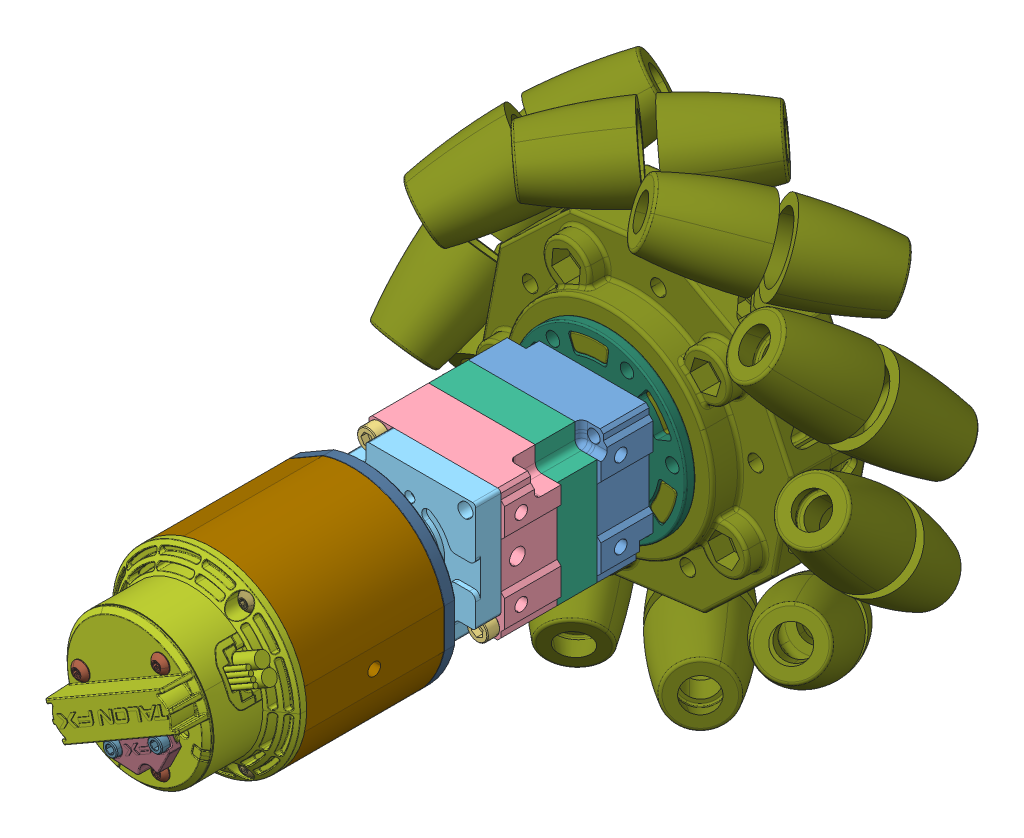
SolidWorks assembly LeftMotorStack, configuration Default. Lengths in mm.
Overall size (198.43 195.51 209.52).
34 component instances, 27 part files, 5 mates.
Components (placement in the parent):
- MotorStack-1: MotorStack [Default] at (-4.3094 29.1715 123.7803) size (81.62 81.39 192.35)
  - v2-VersaPlanetary-1stage-with-AM9015-20131031-1: v2-VersaPlanetary-1stage-with-AM9015-20131031 [Default] at (32.9453 91.261 18.2063) x (0 0 -1) z (0 1 0) size (95.9 44.45 42.1)
    - 217-2625-026 Rev1-1: 217-2625-026 Rev1 [Default] at (-6.5 22.225 0) x (0 -1 0) z (-1 0 0) size (44.45 42 18.13)
    - 217-2742-001 Rev4-1: 217-2742-001 Rev4 [Default] at (0.2002 22.225 0) x (1 0 0) z (0 -0.092627 0.995701) size (7 28 28)
    - 217-2742-001 Rev4-2: 217-2742-001 Rev4 [Default] at (8.2002 22.225 0) size (7 28 28)
    - 217-2625-017 Rev1_9714K61-1: 217-2625-017 Rev1_9714K61 [Default] at (7.42 22.3002 -0.342) x (0 0.56703 0.823697) z (0 -0.823697 0.56703) size (28.51 4.98 30.18)
    - 217-2625-003 Rev1-1: 217-2625-003 Rev1 [Default] at (7.4478 22.225 0) x (0 -1 0) z (1 0 0) size (17 17 64.12)
    - 217-2625-018 Rev1_98541A410-1: 217-2625-018 Rev1_98541A410 [Default] at (-0.7046 22.225 0) x (1 0 0) z (0 -0.017452 0.999848) size (1 19.6 17.4)
    - 832-1750-Ring-Gear-Screw_SSA0832-0500ZC-1: 832-1750-Ring-Gear-Screw_SSA0832-0500ZC [Default] at (-30.7 4.725 -17.5) x (0 0.997447 0.071411) z (0 -0.071411 0.997447) size (6.73 48.51 6.73)
    - 832-1750-Ring-Gear-Screw_SSA0832-0500ZC-2: 832-1750-Ring-Gear-Screw_SSA0832-0500ZC [Default] at (-30.7 39.725 17.5) x (0 0.005929 0.999982) z (0 -0.999982 0.005929) size (6.73 48.51 6.73)
    - 217-2625-025 Rev1-1: 217-2625-025 Rev1 [Default] at (-23.2 22.225 0) x (0 -1 0) z (-1 0 0) size (44.45 42 18)
    - 217-2822-004 Rev4-1: 217-2822-004 Rev4 [Default] at (-37.7 22.225 0) x (0 -1 0) z (-1 0 0) size (42 42 9.8)
    - 217-2820 Rev1_Public-1: 217-2820 Rev1_Public [Default] at (-4.6546 22.225 0) x (0 -0.456494 0.889726) z (-1 0 0)
      - 217-2625-100-1: 217-2625-100 [Default] at origin
    - 217-2816-001 Rev1-1: 217-2816-001 Rev1 [Default] at (-6.35 22.225 0) x (0 -1 0) z (1 0 0) size (42 42 14.5)
    - 217-4649-001 Rev1-1: 217-4649-001 Rev1 [Default] at (-20.046 22.225 0) x (0 -1 0) z (1 0 0) size (18 18 13)
    - 217-4649-007 Rev1_94105A824-1: 217-4649-007 Rev1_94105A824 [Default] at (-25.521 22.225 -6.7835) x (-0.996104 -0.088191 0) z (0 0 -1) size (4.83 4.83 4.9)
    - 217-2625-014 Rev2-1: 217-2625-014 Rev2 [Default] at (-24.7818 22.225 0) x (0 0 1) z (0 -1 0) size (8.01 7.5 7.94)
  - Falcon_500_Powered_by_Talon_FX_217-6515-1: Falcon_500_Powered_by_Talon_FX_217-6515 [Default] at (9.4877 97.4968 108.3478) x (1 0 0) z (0 0 -1) size (81.62 81.39 116.76)
    - Copy of 217-6515-Back 20190920^Falcon_500_Powered_by_Talon_FX_217-6515-1: Copy of 217-6515-Back 20190920^Falcon_500_Powered_by_Talon_FX_217-6515 [Default] at (1.2326 6.2358 -14.9619) size (60.06 60.12 79.55) (virtual)
    - Copy of Copy of 217-6515-201 Rev6^Falcon_500_Powered_by_Talon_FX_217-6515-1: Copy of Copy of 217-6515-201 Rev6^Falcon_500_Powered_by_Talon_FX_217-6515 [Default] at (1.2326 6.2358 50.6381) x (0.809017 0.587785 0) z (0 0 1) size (9.31 9.33 42.21) (virtual)
    - Copy of 217-6515-002 Rev6^Falcon_500_Powered_by_Talon_FX_217-6515-1: Copy of 217-6515-002 Rev6^Falcon_500_Powered_by_Talon_FX_217-6515 [Default] at (1.2326 6.2358 10.7381) x (0 -1 0) z (0 0 1) size (60 59.34 44.4) (virtual)
    - Copy of 217-6515-001 Rev6^Falcon_500_Powered_by_Talon_FX_217-6515-1: Copy of 217-6515-001 Rev6^Falcon_500_Powered_by_Talon_FX_217-6515 [Default] at (1.2326 6.2358 30.9381) x (0.5 0.866025 0) z (0 0 1) size (59.34 59.99 10) (virtual)
    - Copy of M3 BHTS-SECURE, Grade 8 Steel Rev1_SBTM3-24MMZB-SECURE^Falcon_500_Powered_by_Talon_FX_217-6515-1: Copy of M3 BHTS-SECURE, Grade 8 Steel Rev1_SBTM3-24MMZB-SECURE^Falcon_500_Powered_by_Talon_FX_217-6515 [Default] at (9.7324 20.9581 -38.0119) x (-0.923728 -0.383049 0) z (0 0 -1) size (5.69 5.69 25.65) (virtual)
    - Copy (2) of M3 BHTS-SECURE, Grade 8 Steel Rev1_SBTM3-24MMZB-SECURE^Falcon_500_Powered_by_Talon_FX_217-6515-2: Copy (2) of M3 BHTS-SECURE, Grade 8 Steel Rev1_SBTM3-24MMZB-SECURE^Falcon_500_Powered_by_Talon_FX_217-6515 [Default] at (-15.7672 6.2357 -38.0119) x (0.793594 -0.608447 0) z (0 0 -1) size (5.69 5.69 25.65) (virtual)
    - Copy (3) of M3 BHTS-SECURE, Grade 8 Steel Rev1_SBTM3-24MMZB-SECURE^Falcon_500_Powered_by_Talon_FX_217-6515-3: Copy (3) of M3 BHTS-SECURE, Grade 8 Steel Rev1_SBTM3-24MMZB-SECURE^Falcon_500_Powered_by_Talon_FX_217-6515 [Default] at (9.7326 -8.4864 -38.0119) x (0.130134 0.991496 0) z (0 0 -1) size (5.69 5.69 25.65) (virtual)
    - Copy of M3 BHTS, Grade 8 Steel Rev1_SBTM3-50MMZB^Falcon_500_Powered_by_Talon_FX_217-6515-1: Copy of M3 BHTS, Grade 8 Steel Rev1_SBTM3-50MMZB^Falcon_500_Powered_by_Talon_FX_217-6515 [Default] at (14.3576 28.969 -14.8619) x (-0.923728 -0.383049 0) z (0 0 -1) size (5.7 5.7 51.65) (virtual)
    - Copy (2) of M3 BHTS, Grade 8 Steel Rev1_SBTM3-50MMZB^Falcon_500_Powered_by_Talon_FX_217-6515-2: Copy (2) of M3 BHTS, Grade 8 Steel Rev1_SBTM3-50MMZB^Falcon_500_Powered_by_Talon_FX_217-6515 [Default] at (-25.0174 6.2358 -14.8619) x (0.793594 -0.608447 0) z (0 0 -1) size (5.7 5.7 51.65) (virtual)
    - Copy (3) of M3 BHTS, Grade 8 Steel Rev1_SBTM3-50MMZB^Falcon_500_Powered_by_Talon_FX_217-6515-3: Copy (3) of M3 BHTS, Grade 8 Steel Rev1_SBTM3-50MMZB^Falcon_500_Powered_by_Talon_FX_217-6515 [Default] at (14.3576 -16.4974 -14.8619) x (0.130134 0.991496 0) z (0 0 -1) size (5.7 5.7 51.65) (virtual)
    - Copy of 217-6515-308 Rev5^Falcon_500_Powered_by_Talon_FX_217-6515-1: Copy of 217-6515-308 Rev5^Falcon_500_Powered_by_Talon_FX_217-6515 [Default] at (7.0724 16.3512 -38.3619) x (0.866013 -0.500022 0) z (0.500022 0.866013 0) size (21.32 4.25 9.95) (virtual)
    - Copy of #4-40 SHCS, Grade 8 Steel Rev2_SSA0440-0125ZB^Falcon_500_Powered_by_Talon_FX_217-6515-1: Copy of #4-40 SHCS, Grade 8 Steel Rev2_SSA0440-0125ZB^Falcon_500_Powered_by_Talon_FX_217-6515 [Default] at (-1.3722 18.2247 -35.6869) x (-0.90374 0.428082 0) z (0 0 -1) size (4.65 4.65 6.03) (virtual)
    - Copy (2) of #4-40 SHCS, Grade 8 Steel Rev2_SSA0440-0125ZB^Falcon_500_Powered_by_Talon_FX_217-6515-2: Copy (2) of #4-40 SHCS, Grade 8 Steel Rev2_SSA0440-0125ZB^Falcon_500_Powered_by_Talon_FX_217-6515 [Default] at (12.917 9.9744 -35.6869) x (-0.992189 0.124742 0) z (0 0 -1) size (4.65 4.65 6.03) (virtual)
- MechanumHub-1: MechanumHub [Default] at (6.411 120.4326 107.8991) x (0 0 1) z (-0.922976 0.384858 0) size (12.7 55.88 55.88)
- Vex 6in Left-2: Vex 6in Left [Default] at (6.411 120.4326 95.8341) x (0.903597 0.428384 0) z (0 0 1) size (150.41 150.31 56.44)
Mates (geometry in assembly coordinates):
- Concentric3: concentric anti-aligned: circle of MotorStack-1/v2-VersaPlanetary-1stage-with-AM9015-20131031-1/217-2625-026 Rev1-1; cylinder of MechanumHub-1 through (6.411 120.4326 120.5991) axis (0 0 1) radius 14.2949
- Distance1: distance = 4.7625 mm anti-aligned: plane of MotorStack-1/v2-VersaPlanetary-1stage-with-AM9015-20131031-1/217-2625-026 Rev1-1 through (-15.814 142.6576 125.3616) normal (0 0 -1); plane of MechanumHub-1 through (18.552 149.5495 120.5991) normal (0 0 1)
- Concentric4: concentric aligned: cylinder of MechanumHub-1 through (6.411 120.4326 122.1993) axis (0 0 -1) radius 27.94; circle of Vex 6in Left-2
- Coincident1: coincident anti-aligned: plane of MechanumHub-1 through (11.9125 133.6264 117.4241) normal (0 0 -1); plane of Vex 6in Left-2 through (6.411 120.4326 117.4241) normal (0 0 1)
- Concentric5: concentric anti-aligned: circle of MechanumHub-1; cylinder of Vex 6in Left-2 through (-17.2051 117.38 114.2491) axis (0 0 1) radius 2.1526
